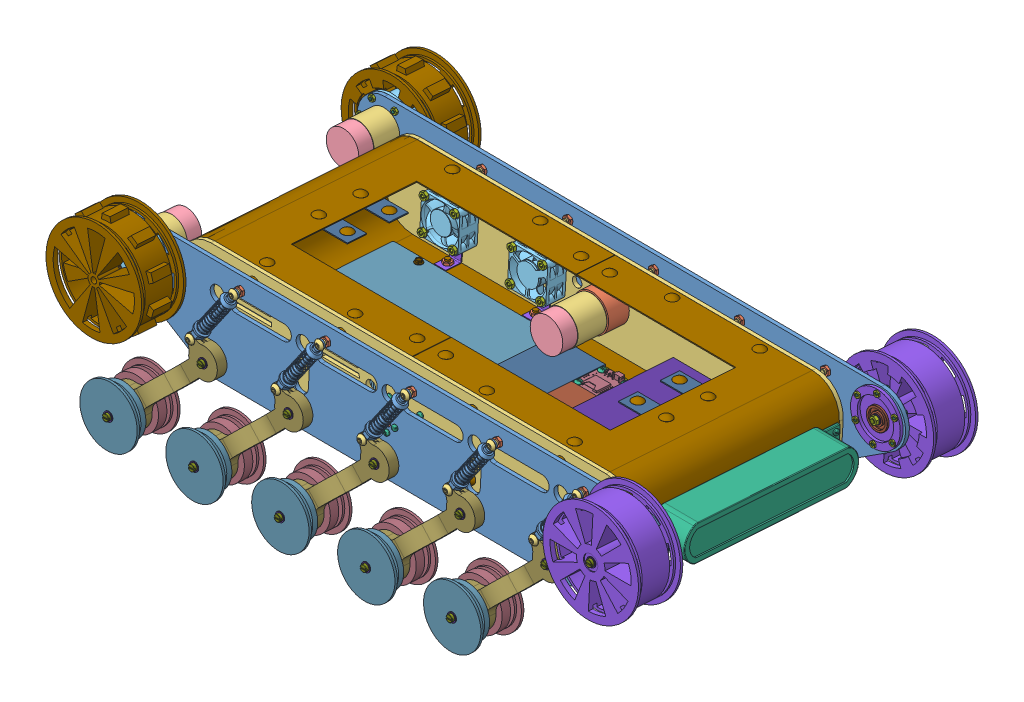
SolidWorks assembly Ensamble_Detallado_2, configuration Predeterminado. Lengths in mm.
Overall size (769.79 225.93 366.19).
522 component instances, 48 part files, 262 mates.
Components (placement in the parent):
- Perfil_IzquierdoV2.2-1: Perfil_IzquierdoV2.2 [Predeterminado] at (68.4496 -9.6253 -539.9326) x (0.999983 -0.000205 0.005895) z (-0.005872 0.060029 0.998179) size (574.48 100.85 4)
- Motor_4-1: Motor_4 [Predeterminado] at (-189.8361 39.4073 -564.1867) x (0.999983 -0.000205 0.005895) z (-0.005872 0.060029 0.998179) size (43.61 43.61 89.6)
  - Motor_1-1: Motor_1 [Predeterminado] at (-1.5658 -18.1483 21.75) size (36.8 36.8 43.5)
  - Motor_2-1: Motor_2 [Predeterminado] at (-1.5658 -18.1483 -8.95) x (-0.954241 0.299039 0) z (0 0 1) size (34.8 34.8 30.7)
  - Motor_3-1: Motor_3 [Predeterminado] at (-1.5658 -18.1483 -24.35) x (0.996313 -0.085794 0) z (0 0 1) size (34 34 15.4)
- Tapa_motor-1: Tapa_motor [Predeterminado] at (-191.6836 24.0684 -516.9408) x (-0.999983 0.000205 -0.005895) z (0.005872 -0.060029 -0.998179) size (54.48 54.48 24.5)
- pan head tapping screw_am-8: pan head tapping screw_am [PHT 3x6x5.5-slot-D-N] at (-183.9391 37.598 -515.5049) x (0.005872 -0.060029 -0.998179) z (-0.134849 -0.989126 0.058691) size (8.2 5.6 5.6)
- pan head tapping screw_am-9: pan head tapping screw_am [PHT 3x6x5.5-slot-D-N] at (-176.1968 24.1972 -514.6534) x (0.005872 -0.060029 -0.998179) z (-0.925525 -0.378291 0.017305) size (8.2 5.6 5.6)
- pan head tapping screw_am-10: pan head tapping screw_am [PHT 3x6x5.5-slot-D-N] at (-183.9541 10.7996 -513.8933) x (0.005872 -0.060029 -0.998179) z (-0.790675 0.610835 -0.041386) size (8.2 5.6 5.6)
- pan head tapping screw_am-11: pan head tapping screw_am [PHT 3x6x5.5-slot-D-N] at (-199.4539 10.8028 -513.9847) x (0.005872 -0.060029 -0.998179) z (0.134849 0.989126 -0.058691) size (8.2 5.6 5.6)
- pan head tapping screw_am-12: pan head tapping screw_am [PHT 3x6x5.5-slot-D-N] at (-207.1962 24.2036 -514.8361) x (0.005872 -0.060029 -0.998179) z (0.925525 0.378291 -0.017305) size (8.2 5.6 5.6)
- pan head tapping screw_am-13: pan head tapping screw_am [PHT 3x6x5.5-slot-D-N] at (-199.4389 37.6012 -515.5962) x (0.005872 -0.060029 -0.998179) z (0.790675 -0.610835 0.041386) size (8.2 5.6 5.6)
- pan head tapping screw_am-14: pan head tapping screw_am [PHT 3x10x9-slot-D-N] at (-215.3099 22.8964 -536.3445) x (0.005872 -0.060029 -0.998179) z (0.809274 0.586638 -0.030519) size (12.2 5.6 5.6)
- hex nut style 1_am-1: hex nut style 1_am [B18.2.4.1M - Hex nut, Style 1,  M3 x 0.5 --D-N] at (-215.2558 22.3441 -545.5277) x (0.970127 -0.241753 0.020245) z (-0.005872 0.060029 0.998179) size (5.5 6.35 2.4)
- Pieza_Fijacion-1: Pieza_Fijacion [Predeterminado] at (328.1431 22.6984 -545.358) x (0.999454 -0.032109 0.00781) z (0.005872 -0.060029 -0.998179) size (52 52 4)
- pan head tapping screw_am-20: pan head tapping screw_am [PHT 3x10x9-slot-D-N] at (328.8149 45.7585 -536.5222) x (0.005872 -0.060029 -0.998179) z (0.852997 -0.520651 0.036329) size (12.2 5.6 5.6)
- hex nut style 1_am-7: hex nut style 1_am [B18.2.4.1M - Hex nut, Style 1,  M3 x 0.5 --D-N] at (328.8748 45.1462 -546.7037) x (-0.437994 -0.897507 0.051398) z (-0.005872 0.060029 0.998179) size (5.5 6.35 2.4)
- Ensamble_internoV1.1-1: Ensamble_internoV1.1 [Predeterminado] at (-380.1452 -33.1767 -776.9821) x (0.005872 -0.060029 -0.998179) z (0.999983 0.000382 0.005859) size (210 91 474)
  - ChasisV1.7-1: ChasisV1.7 [Predeterminado] at (-114.8477 22.7516 450) size (210 84 474)
  - roboclaw-1: roboclaw [Predeterminado] at (-157.9377 -17.2484 439.18) x (1 0 0) z (0 1 0) size (74 52 2)
  - roboclaw-3: roboclaw [Predeterminado] at (-61.7577 -17.2484 439.18) x (-1 0 0) z (0 1 0) size (74 52 2)
  - Regulador-1: Regulador [Predeterminado] at (-109.8477 -17.2484 499.18) x (-1 0 0) z (0 1 0) size (100 68 2)
  - Conmutador-1: Conmutador [Predeterminado] at (-174.0717 -17.2484 490.58) x (0 0 1) z (0 1 0) size (50.8 28.45 2)
  - imu-1: imu [Default] at (-43.9727 -15.9784 481.055) x (-1 0 0) z (0 0 1) size (31.75 5.84 31.75)
  - jetson-1: jetson [Predeterminado] at (-188.5877 -15.6734 408.1) x (1 0 0) z (0 1 0) size (170.18 170.18 1.57)
  - lipo_holder-1: lipo_holder [Predeterminado] at (-109.8477 -18.2484 627) x (0 0 -1) z (0 1 0) size (60 185 60)
  - Plastico-1: Plastico [Predeterminado] at (-109.8477 -18.2484 388.09) x (1 0 0) z (0 1 0) size (170.18 290.18 1)
  - lipo_holder-2: lipo_holder [Predeterminado] at (-109.8477 -18.2484 567) x (0 0 -1) z (0 1 0) size (60 185 60)
  - batería-1: batería [Predeterminado] at (-32.3477 -14.2484 604) x (0 1 0) z (0 0 1) size (48 152 48)
  - batería-2: batería [Predeterminado] at (-35.3477 -14.2484 544) x (0 1 0) z (0 0 1) size (48 152 48)
  - hex flange head tapping screw_am-1: hex flange head tapping screw_am [HEXFHTS 3.5x8x6.7-Indented head-AB-N] at (-31.1077 -15.6734 276.02) x (0 -1 0) z (0 0 1) size (10.9 7.5 7.5)
  - hex flange head tapping screw_am-2: hex flange head tapping screw_am [HEXFHTS 3.5x8x6.7-Indented head-AB-N] at (-188.5877 -15.6734 253.18) x (0 -1 0) z (0 0 1) size (10.9 7.5 7.5)
  - hex flange head tapping screw_am-3: hex flange head tapping screw_am [HEXFHTS 3.5x8x6.7-Indented head-AB-N] at (-188.5877 -15.6734 408.1) x (0 -1 0) z (0 0 1) size (10.9 7.5 7.5)
  - hex flange head tapping screw_am-4: hex flange head tapping screw_am [HEXFHTS 3.5x8x6.7-Indented head-AB-N] at (-31.1077 -15.6734 408.1) x (0 -1 0) z (0 0 1) size (10.9 7.5 7.5)
  - prevailing torque hex nut_am-1: prevailing torque hex nut_am [AM-M3.5-N] at (-31.1077 -22.7484 276.02) x (1 0 0) z (0 -1 0) size (6 7.33 3.5)
  - prevailing torque hex nut_am-2: prevailing torque hex nut_am [AM-M3.5-N] at (-188.5877 -22.7484 253.18) x (1 0 0) z (0 -1 0) size (6 7.33 3.5)
  - prevailing torque hex nut_am-3: prevailing torque hex nut_am [AM-M3.5-N] at (-31.1077 -22.7484 408.1) x (1 0 0) z (0 -1 0) size (6 7.33 3.5)
  - prevailing torque hex nut_am-4: prevailing torque hex nut_am [AM-M3.5-N] at (-188.5877 -22.7484 408.1) x (0.006529 0 -0.999979) z (0 -1 0) size (6 7.33 3.5)
  - pan head tapping screw_am-1: pan head tapping screw_am [PHT 4.2x8x6.6-slot-AB-N] at (-31.7377 -14.1484 493.29) x (0 -1 0) z (0 0 1) size (11.21 7 7)
  - pan head tapping screw_am-2: pan head tapping screw_am [PHT 4.2x8x6.6-slot-AB-N] at (-56.2081 -15.1484 493.2904) x (0 -1 0) z (0 0 1) size (11.21 7 7)
  - pan head tapping screw_am-4: pan head tapping screw_am [PHT 4.2x8x6.6-slot-AB-N] at (-56.2077 -14.1484 468.82) x (0 -1 0) z (0 0 1) size (11.21 7 7)
  - pan head tapping screw_am-5: pan head tapping screw_am [PHT 4.2x8x6.6-slot-AB-N] at (-31.7377 -14.1484 468.82) x (0 -1 0) z (0 0 1) size (11.21 7 7)
  - hex nut jam_am-3: hex nut jam_am [B18.2.4.5M - Hex jam nut,  M5 x 0.8 --D-N] at (-31.7377 -19.2484 493.29) x (0.998096 0 -0.061678) z (0 1 0) size (8 9.24 2.7)
  - hex nut jam_am-4: hex nut jam_am [B18.2.4.5M - Hex jam nut,  M5 x 0.8 --D-N] at (-56.2081 -21.9484 493.2904) x (0 0 -1) z (0 -1 0) size (8 9.24 2.7)
  - hex nut jam_am-5: hex nut jam_am [B18.2.4.5M - Hex jam nut,  M5 x 0.8 --D-N] at (-31.7377 -21.9484 468.82) x (1 0 0) z (0 -1 0) size (8 9.24 2.7)
  - hex nut jam_am-6: hex nut jam_am [B18.2.4.5M - Hex jam nut,  M5 x 0.8 --D-N] at (-56.2077 -21.9484 468.82) x (0 0 -1) z (0 -1 0) size (8 9.24 2.7)
  - socket button head cap screw_am-3: socket button head cap screw_am [B18.3.4M - 4 x 0.7 x 8 SBHCS --N] at (-22.3477 -12.0484 617) x (0 -1 0) z (-0.458504 0 0.888692) size (10.2 7.6 7.6)
  - socket button head cap screw_am-4: socket button head cap screw_am [B18.3.4M - 4 x 0.7 x 8 SBHCS --N] at (-22.3477 -12.0484 557) x (0 -1 0) z (-0.211914 0 0.977288) size (10.2 7.6 7.6)
  - socket button head cap screw_am-5: socket button head cap screw_am [B18.3.4M - 4 x 0.7 x 8 SBHCS --N] at (-22.3477 -12.0484 576.6022) x (0 -1 0) z (-0.545234 0 0.838284) size (10.2 7.6 7.6)
  - socket button head cap screw_am-6: socket button head cap screw_am [B18.3.4M - 4 x 0.7 x 8 SBHCS --N] at (-22.3477 -12.0484 636.6022) x (0 -1 0) z (-0.646269 0 0.76311) size (10.2 7.6 7.6)
  - hex thin nut gradeb_din-1: hex thin nut gradeb_din [Hexagon Nut ISO 4036 - M4 - N] at (-22.3477 -19.4976 636.6022) x (1 0 0) z (0 1 0) size (7 8.08 2.2)
  - hex thin nut gradeb_din-2: hex thin nut gradeb_din [Hexagon Nut ISO 4036 - M4 - N] at (-22.3477 -19.6363 617) x (1 0 0) z (0 1 0) size (7 8.08 2.2)
  - hex thin nut gradeb_din-3: hex thin nut gradeb_din [Hexagon Nut ISO 4036 - M4 - N] at (-147.9786 -8.1538 555.9748) size (7 8.08 2.2)
  - hex thin nut gradeb_din-4: hex thin nut gradeb_din [Hexagon Nut ISO 4036 - M4 - N] at (-22.3477 -21.4484 557) x (-0.957833 0 0.287325) z (0 -1 0) size (7 8.08 2.2)
  - hex thin nut gradeb_din-5: hex thin nut gradeb_din [Hexagon Nut ISO 4036 - M4 - N] at (-22.3477 -19.2484 576.6022) x (0.99798 0 0.063529) z (0 1 0) size (7 8.08 2.2)
  - socket button head cap screw_am-8: socket button head cap screw_am [B18.3.4M - 4 x 0.7 x 8 SBHCS --N] at (-197.3477 -12.0484 557) x (0 -1 0) z (-0.211914 0 -0.977288) size (10.2 7.6 7.6)
  - socket button head cap screw_am-9: socket button head cap screw_am [B18.3.4M - 4 x 0.7 x 8 SBHCS --N] at (-197.3477 -12.0484 576.6022) x (0 -1 0) z (-0.545234 0 -0.838284) size (10.2 7.6 7.6)
  - socket button head cap screw_am-10: socket button head cap screw_am [B18.3.4M - 4 x 0.7 x 8 SBHCS --N] at (-197.3477 -12.0484 617) x (0 -1 0) z (-0.458504 0 -0.888692) size (10.2 7.6 7.6)
  - socket button head cap screw_am-11: socket button head cap screw_am [B18.3.4M - 4 x 0.7 x 8 SBHCS --N] at (-197.3477 -12.0484 636.6022) x (0 -1 0) z (-0.646269 0 -0.76311) size (10.2 7.6 7.6)
  - hex thin nut gradeb_din-6: hex thin nut gradeb_din [Hexagon Nut ISO 4036 - M4 - N] at (-197.3477 -21.4484 576.6022) x (-0.99798 0 0.063529) z (0 -1 0) size (7 8.08 2.2)
  - hex thin nut gradeb_din-7: hex thin nut gradeb_din [Hexagon Nut ISO 4036 - M4 - N] at (-197.3477 -19.2484 557) x (0.957833 0 0.287325) z (0 1 0) size (7 8.08 2.2)
  - hex thin nut gradeb_din-8: hex thin nut gradeb_din [Hexagon Nut ISO 4036 - M4 - N] at (-197.3477 -21.8363 617) x (-1 0 0) z (0 -1 0) size (7 8.08 2.2)
  - hex thin nut gradeb_din-9: hex thin nut gradeb_din [Hexagon Nut ISO 4036 - M4 - N] at (-197.3477 -21.6976 636.6022) x (-1 0 0) z (0 -1 0) size (7 8.08 2.2)
- fan-1: fan [По умолчанию] at (0.0753 3.2018 -561.6937) x (-0.999983 -0.000176 -0.005872) z (0.005872 -0.060029 -0.998179) size (41.13 41.33 20.18)
- fan-2: fan [По умолчанию] at (-91.8057 2.0201 -582.1996) x (0.999983 0.000176 0.005872) z (-0.005872 0.060029 0.998179) size (41.13 41.33 20.18)
- Soporte_zed-1: Soporte_zed [Predeterminado] at (340.1967 -3.5969 -664.4756) x (-0.005872 0.060029 0.998179) z (-0.999983 -0.000382 -0.005859) size (205.99 36.47 36.01)
- hex nut style 1 gradeab_bsi-1: hex nut style 1 gradeab_bsi [BS EN 24032 - M4 - W - N] at (-107.8026 17.9884 -583.254) x (0.99528 -0.096345 0.011649) z (-0.005872 0.060029 0.998179) size (7 8.08 3.2)
- hex nut style 1 gradeab_bsi-2: hex nut style 1 gradeab_bsi [BS EN 24032 - M4 - W - N] at (-107.7894 -14.1459 -584.5273) x (-0.581467 -0.8123 0.04543) z (0.005872 -0.060029 -0.998179) size (7 8.08 3.2)
- hex nut style 1 gradeab_bsi-3: hex nut style 1 gradeab_bsi [BS EN 24032 - M4 - W - N] at (-75.79 -14.1403 -584.3394) x (-0.984097 0.176868 -0.016425) z (0.005872 -0.060029 -0.998179) size (7 8.08 3.2)
- hex nut style 1 gradeab_bsi-4: hex nut style 1 gradeab_bsi [BS EN 24032 - M4 - W - N] at (-75.7843 17.802 -586.2603) x (-0.58545 0.809033 -0.052098) z (0.005872 -0.060029 -0.998179) size (7 8.08 3.2)
- hex nut style 1 gradeab_bsi-5: hex nut style 1 gradeab_bsi [BS EN 24032 - M4 - W - N] at (-15.7854 17.7775 -585.9059) x (-0.58545 0.809033 -0.052098) z (0.005872 -0.060029 -0.998179) size (7 8.08 3.2)
- hex nut style 1 gradeab_bsi-6: hex nut style 1 gradeab_bsi [BS EN 24032 - M4 - W - N] at (-15.791 -14.1648 -583.985) x (0.609484 0.791576 -0.044019) z (0.005872 -0.060029 -0.998179) size (7 8.08 3.2)
- hex nut style 1 gradeab_bsi-7: hex nut style 1 gradeab_bsi [BS EN 24032 - M4 - W - N] at (16.2141 17.7832 -585.718) x (-0.984097 0.176868 -0.016425) z (0.005872 -0.060029 -0.998179) size (7 8.08 3.2)
- hex nut style 1 gradeab_bsi-8: hex nut style 1 gradeab_bsi [BS EN 24032 - M4 - W - N] at (16.2084 -14.1591 -583.7971) x (0.609484 0.791576 -0.044019) z (0.005872 -0.060029 -0.998179) size (7 8.08 3.2)
- Pieza_union_chasis-1: Pieza_union_chasis [Predeterminado] at (-92.4935 43.6291 -564.6695) x (-0.999983 -0.000382 -0.005859) z (0.005872 -0.060029 -0.998179) size (12 20 17)
- round head bolt_ai-8: round head bolt_ai [RHBOLT 0.19-24x0.25x0.25-N] at (-92.3708 46.562 -573.8615) x (0.000029 -0.998197 0.06003) z (-0.000001 0.06003 0.998197) size (8.99 11.53 11.53)
- hex nut jam_am-6: hex nut jam_am [B18.2.4.5M - Hex jam nut,  M5 x 0.8 --D-N] at (-92.3707 42.0907 -573.5926) x (0.997706 0.004093 0.067568) z (-0.000029 0.998197 -0.06003) size (8 9.24 2.7)
- round head bolt_ai-9: round head bolt_ai [RHBOLT 0.19-24x0.25x0.25-N] at (-92.5322 32.0495 -557.3196) x (0.005872 -0.060029 -0.998179) z (0 -0.998197 0.06003) size (8.99 11.53 11.53)
- hex nut jam_am-7: hex nut jam_am [B18.2.4.5M - Hex jam nut,  M5 x 0.8 --D-N] at (-92.4715 31.4287 -567.6424) x (0.997689 0.06792 0.001784) z (0.005872 -0.060029 -0.998179) size (8 9.24 2.7)
- hex nut jam_am-10: hex nut jam_am [B18.2.4.5M - Hex jam nut,  M5 x 0.8 --D-N] at (-0.3831 31.4638 -567.1028) x (0.997689 0.06792 0.001784) z (0.005872 -0.060029 -0.998179) size (8 9.24 2.7)
- round head bolt_ai-12: round head bolt_ai [RHBOLT 0.19-24x0.25x0.25-N] at (-0.4438 32.0846 -556.78) x (0.005872 -0.060029 -0.998179) z (0 -0.998197 0.06003) size (8.99 11.53 11.53)
- Pieza_union_chasis-3: Pieza_union_chasis [Predeterminado] at (-0.4051 43.6643 -564.1299) x (-0.999983 -0.000382 -0.005859) z (0.005872 -0.060029 -0.998179) size (12 20 17)
- round head bolt_ai-13: round head bolt_ai [RHBOLT 0.19-24x0.25x0.25-N] at (-0.2824 46.5972 -573.3219) x (0.000029 -0.998197 0.06003) z (-0.000001 0.06003 0.998197) size (8.99 11.53 11.53)
- hex nut jam_am-11: hex nut jam_am [B18.2.4.5M - Hex jam nut,  M5 x 0.8 --D-N] at (-0.2823 42.1259 -573.0531) x (0.997706 0.004093 0.067568) z (-0.000029 0.998197 -0.06003) size (8 9.24 2.7)
- Pieza_union_chasis-4: Pieza_union_chasis [Predeterminado] at (137.5925 43.636 -563.3164) x (-0.999983 -0.000382 -0.005859) z (0.005872 -0.060029 -0.998179) size (12 20 17)
- round head bolt_ai-14: round head bolt_ai [RHBOLT 0.19-24x0.25x0.25-N] at (137.5538 32.0564 -555.9666) x (0.005872 -0.060029 -0.998179) z (0 -0.998197 0.06003) size (8.99 11.53 11.53)
- hex nut jam_am-12: hex nut jam_am [B18.2.4.5M - Hex jam nut,  M5 x 0.8 --D-N] at (137.6145 31.4356 -566.2893) x (0.997689 0.06792 0.001784) z (0.005872 -0.060029 -0.998179) size (8 9.24 2.7)
- round head bolt_ai-15: round head bolt_ai [RHBOLT 0.19-24x0.25x0.25-N] at (137.7152 46.5689 -572.5085) x (0.000029 -0.998197 0.06003) z (-0.000001 0.06003 0.998197) size (8.99 11.53 11.53)
- hex nut jam_am-13: hex nut jam_am [B18.2.4.5M - Hex jam nut,  M5 x 0.8 --D-N] at (137.7153 42.0976 -572.2396) x (0.997706 0.004093 0.067568) z (-0.000029 0.998197 -0.06003) size (8 9.24 2.7)
- Puerta-1: Puerta [Predeterminado] at (69.2002 37.2257 -668.5247) x (0.005872 -0.060029 -0.998179) z (-0.000029 0.998197 -0.06003) size (130 334 1) (hidden)
- lamina_union-2: lamina_union [Predeterminado] at (236.0701 38.5901 -645.919) x (-0.005872 0.060029 0.998179) z (0.000029 -0.998197 0.06003) size (20 50 1)
- lamina_union-3: lamina_union [Predeterminado] at (68.7011 41.33 -583.6195) x (0.005872 -0.060029 -0.998179) z (-0.000029 0.998197 -0.06003) size (20 50 1)
- lamina_union-4: lamina_union [Predeterminado] at (-97.9242 38.4626 -647.876) x (-0.005872 0.060029 0.998179) z (0.000029 -0.998197 0.06003) size (20 50 1)
- round head bolt_ai-26: round head bolt_ai [RHBOLT 0.19-24x0.25x0.25-N] at (-112.924 42.0919 -648.1825) x (0.000029 -0.998197 0.06003) z (-0.000001 0.06003 0.998197) size (8.99 11.53 11.53)
- hex nut jam_am-24: hex nut jam_am [B18.2.4.5M - Hex jam nut,  M5 x 0.8 --D-N] at (251.0698 37.5976 -645.7711) x (0.997706 0.004093 0.067568) z (-0.000029 0.998197 -0.06003) size (8 9.24 2.7)
- round head bolt_ai-27: round head bolt_ai [RHBOLT 0.19-24x0.25x0.25-N] at (-82.9245 42.1033 -648.0067) x (0.000029 -0.998197 0.06003) z (-0.000001 0.06003 0.998197) size (8.99 11.53 11.53)
- round head bolt_ai-28: round head bolt_ai [RHBOLT 0.19-24x0.25x0.25-N] at (83.7007 45.9689 -583.8102) x (0.000029 -0.998197 0.06003) z (-0.000001 0.06003 0.998197) size (8.99 11.53 11.53)
- round head bolt_ai-29: round head bolt_ai [RHBOLT 0.19-24x0.25x0.25-N] at (221.0702 42.2194 -646.2255) x (0.000029 -0.998197 0.06003) z (-0.000001 0.06003 0.998197) size (8.99 11.53 11.53)
- round head bolt_ai-30: round head bolt_ai [RHBOLT 0.19-24x0.25x0.25-N] at (251.0697 42.2309 -646.0497) x (0.000029 -0.998197 0.06003) z (-0.000001 0.06003 0.998197) size (8.99 11.53 11.53)
- round head bolt_ai-31: round head bolt_ai [RHBOLT 0.19-24x0.25x0.25-N] at (53.7012 45.9575 -583.986) x (0.000029 -0.998197 0.06003) z (-0.000001 0.06003 0.998197) size (8.99 11.53 11.53)
- hex nut jam_am-25: hex nut jam_am [B18.2.4.5M - Hex jam nut,  M5 x 0.8 --D-N] at (-112.9239 37.4586 -647.9039) x (0.924389 -0.022871 -0.380764) z (-0.000029 0.998197 -0.06003) size (8 9.24 2.7)
- hex nut jam_am-26: hex nut jam_am [B18.2.4.5M - Hex jam nut,  M5 x 0.8 --D-N] at (83.7008 41.3357 -583.5316) x (0.642396 -0.045986 -0.764992) z (-0.000029 0.998197 -0.06003) size (8 9.24 2.7)
- hex nut jam_am-27: hex nut jam_am [B18.2.4.5M - Hex jam nut,  M5 x 0.8 --D-N] at (53.7014 41.3242 -583.7074) x (0.987847 0.00936 0.155149) z (-0.000029 0.998197 -0.06003) size (8 9.24 2.7)
- hex nut jam_am-28: hex nut jam_am [B18.2.4.5M - Hex jam nut,  M5 x 0.8 --D-N] at (221.0704 37.5862 -645.9469) x (0.944813 0.019694 0.327016) z (-0.000029 0.998197 -0.06003) size (8 9.24 2.7)
- hex nut jam_am-29: hex nut jam_am [B18.2.4.5M - Hex jam nut,  M5 x 0.8 --D-N] at (-82.9244 37.4701 -647.7281) x (0.961929 0.016435 0.272807) z (-0.000029 0.998197 -0.06003) size (8 9.24 2.7)
- instrument ball bearing_68_am-5: instrument ball bearing_68_am [AFBMA 12.1.4.1 - 0080-22 - 8,SI,NC,8_68] at (188.8254 -92.4717 -505.6903) x (0.005872 -0.060029 -0.998179) z (0.436634 -0.897859 0.056564) size (7 22 22)
- Pieza_ResorteV1.5-6: Pieza_ResorteV1.5 [Predeterminado] at (188.8254 -92.4717 -505.6903) x (-0.005872 0.060029 0.998179) z (-0.699298 -0.713776 0.038812) size (30 44.97 120)
- Rueda_Resorte2V1.3-13: Rueda_Resorte2V1.3 [Predeterminado] at (188.8548 -92.7718 -510.6812) x (-0.998179 -0.060274 -0.002247) z (0.005872 -0.060029 -0.998179) size (60 60 20.5)
- Rueda_ResorteV1.3-17: Rueda_ResorteV1.3 [Predeterminado] at (188.7961 -92.1715 -500.6994) x (-0.99968 0.024219 -0.007337) z (-0.005872 0.060029 0.998179) size (60 60 17)
- Pasador-1: Pasador [Predeterminado] at (188.9664 -93.9124 -529.6466) x (0.998179 0.060274 0.002247) z (-0.005872 0.060029 0.998179) size (8 8 44.5)
- cheese head screw_as-2: cheese head screw_as [AS-NZS 1427 CH - M4 x 50-N] at (188.6851 -91.037 -481.8338) x (0.005872 -0.060029 -0.998179) z (-0.998179 -0.060274 -0.002247) size (52.62 7 7)
- plain washer - normal_as-1: plain washer - normal_as [AS 1237.1 N - 4] at (188.9711 -93.9604 -530.4452) x (-0.998179 -0.060274 -0.002247) z (0.005872 -0.060029 -0.998179) size (9 9 0.8)
- hex nut style 1_am-62: hex nut style 1_am [B18.2.4.1M - Hex nut, Style 1,  M4 x 0.7 --D-N] at (188.9899 -94.1525 -533.6393) x (-0.998179 -0.060274 -0.002247) z (0.005872 -0.060029 -0.998179) size (7 8.08 3.2)
- plain washer - normal_as-2: plain washer - normal_as [AS 1237.1 N - 4] at (188.7051 -91.2411 -485.2276) x (-0.998179 -0.060274 -0.002247) z (0.005872 -0.060029 -0.998179) size (9 9 0.8)
- Pieza_Resorte_2V1.5-1: Pieza_Resorte_2V1.5 [Predeterminado] at (190.6345 -110.9665 -813.2294) x (0.005872 -0.060029 -0.998179) z (-0.699298 -0.713776 0.038812) size (30 44.97 120)
- cheese head screw_as-3: cheese head screw_as [AS-NZS 1427 CH - M4 x 50-N] at (190.7748 -112.4012 -837.0859) x (-0.005872 0.060029 0.998179) z (-0.99997 -0.005414 -0.005557) size (52.62 7 7)
- hex nut style 1_am-63: hex nut style 1_am [B18.2.4.1M - Hex nut, Style 1,  M4 x 0.7 --D-N] at (190.4889 -109.4778 -788.4745) x (-0.99997 -0.005414 -0.005557) z (0.005872 -0.060029 -0.998179) size (7 8.08 3.2)
- plain washer - normal_as-3: plain washer - normal_as [AS 1237.1 N - 4] at (190.4936 -109.5258 -789.2731) x (-0.99997 -0.005414 -0.005557) z (0.005872 -0.060029 -0.998179) size (9 9 0.8)
- Pasador-2: Pasador [Predeterminado] at (190.7549 -112.1971 -833.692) x (0.999795 0.019701 0.004696) z (-0.005872 0.060029 0.998179) size (8 8 44.5)
- instrument ball bearing_68_am-6: instrument ball bearing_68_am [AFBMA 12.1.4.1 - 0080-22 - 8,SI,NC,8_68] at (190.6345 -110.9665 -813.2294) x (0.005872 -0.060029 -0.998179) z (0.386524 -0.920477 0.05763) size (7 22 22)
- plain washer - normal_as-4: plain washer - normal_as [AS 1237.1 N - 4] at (190.7596 -112.2451 -834.4906) x (-0.99997 -0.005414 -0.005557) z (0.005872 -0.060029 -0.998179) size (9 9 0.8)
- instrument ball bearing_68_am-7: instrument ball bearing_68_am [AFBMA 12.1.4.1 - 0080-22 - 8,SI,NC,8_68] at (249.9398 -48.9149 -793.5702) x (-0.005872 0.060029 0.998179) z (-0.454454 -0.88932 0.050809) size (7 22 22)
- Resorte-1: Resorte [Predeterminado] at (241.4602 -8.2795 -530.4803) x (-0.827134 0.560678 -0.038584) z (-0.561974 -0.825855 0.04636) size (14 14 75.95)
- Resorte-2: Resorte [Predeterminado] at (243.0344 -24.3732 -798.0922) x (-0.827134 0.560678 -0.038584) z (-0.561974 -0.825855 0.04636) size (14 14 75.95)
- socket button head cap screw_am-5: socket button head cap screw_am [B18.3.4M - 5 x 0.8 x 10 SBHCS --N] at (235.7742 -35.5745 -805.2254) x (-0.005872 0.060029 0.998179) z (-0.100585 -0.993169 0.059136) size (12.75 9.5 9.5)
- socket button head cap screw_am-6: socket button head cap screw_am [B18.3.4M - 5 x 0.8 x 10 SBHCS --N] at (234.109 -18.5503 -522.1418) x (0.005872 -0.060029 -0.998179) z (-0.163306 0.984738 -0.060181) size (12.75 9.5 9.5)
- Motor_4-2: Motor_4 [Predeterminado] at (67.8778 18.2739 -605.5302) x (0.994997 0.099904 -0.000155) z (-0.005872 0.060029 0.998179) size (43.61 43.61 89.6)
  - Motor_1-1: Motor_1 [Predeterminado] at (-1.5658 -18.1483 21.75) size (36.8 36.8 43.5)
  - Motor_2-1: Motor_2 [Predeterminado] at (-1.5658 -18.1483 -8.95) x (-0.954241 0.299039 0) z (0 0 1) size (34.8 34.8 30.7)
  - Motor_3-1: Motor_3 [Predeterminado] at (-1.5658 -18.1483 -24.35) x (0.996313 -0.085794 0) z (0 0 1) size (34 34 15.4)
- Acople-1: Acople [Predeterminado] at (68.465 -3.1497 -542.3256) x (0.999983 -0.000205 0.005895) z (0.005872 -0.060029 -0.998179) size (22 22 12)
- Pared_chasis-2: Pared_chasis [Predeterminado] at (68.5756 -1.2687 -561.0219) x (0.999983 -0.000205 0.005895) z (-0.005872 0.060029 0.998179) size (474 84 4)
- pan head tapping screw_am-43: pan head tapping screw_am [PHT 3x10x9-slot-D-N] at (76.0451 16.9329 -555.8613) x (0.005872 -0.060029 -0.998179) z (-0.866854 -0.497942 0.024846) size (12.2 5.6 5.6)
- pan head tapping screw_am-44: pan head tapping screw_am [PHT 3x10x9-slot-D-N] at (76.4285 -2.7792 -536.0897) x (0.005872 -0.060029 -0.998179) z (-0.866854 -0.497942 0.024846) size (12.2 5.6 5.6)
- pan head tapping screw_am-45: pan head tapping screw_am [PHT 3x10x9-slot-D-N] at (59.91 17.0865 -555.9654) x (0.005872 -0.060029 -0.998179) z (-0.00169 -0.998196 0.06002) size (12.2 5.6 5.6)
- pan head tapping screw_am-46: pan head tapping screw_am [PHT 3x10x9-slot-D-N] at (51.7043 3.2148 -555.1795) x (0.005872 -0.060029 -0.998179) z (0.865164 -0.500253 0.035174) size (12.2 5.6 5.6)
- pan head tapping screw_am-47: pan head tapping screw_am [PHT 3x10x9-slot-D-N] at (59.6337 -10.8105 -554.2894) x (0.005872 -0.060029 -0.998179) z (0.866854 0.497942 -0.024846) size (12.2 5.6 5.6)
- pan head tapping screw_am-48: pan head tapping screw_am [PHT 3x10x9-slot-D-N] at (75.7688 -10.9641 -554.1852) x (0.005872 -0.060029 -0.998179) z (0.00169 0.998196 -0.06002) size (12.2 5.6 5.6)
- pan head tapping screw_am-49: pan head tapping screw_am [PHT 3x10x9-slot-D-N] at (83.9745 2.9076 -554.9712) x (0.005872 -0.060029 -0.998179) z (-0.865164 0.500253 -0.035174) size (12.2 5.6 5.6)
- pan head tapping screw_am-50: pan head tapping screw_am [PHT 3x10x9-slot-D-N] at (68.4331 5.208 -536.6171) x (0.005872 -0.060029 -0.998179) z (0.498527 -0.86513 0.05496) size (12.2 5.6 5.6)
- pan head tapping screw_am-51: pan head tapping screw_am [PHT 3x10x9-slot-D-N] at (60.4287 -2.7759 -536.1841) x (0.005872 -0.060029 -0.998179) z (0.866854 0.497942 -0.024846) size (12.2 5.6 5.6)
- pan head tapping screw_am-52: pan head tapping screw_am [PHT 3x10x9-slot-D-N] at (68.4241 -10.7631 -535.6567) x (0.005872 -0.060029 -0.998179) z (-0.498527 0.86513 -0.05496) size (12.2 5.6 5.6)
- hex nut style 1_am-64: hex nut style 1_am [B18.2.4.1M - Hex nut, Style 1,  M3 x 0.5 --D-N] at (76.4766 -3.2714 -544.2748) x (-0.695099 -0.717851 0.039081) z (-0.005872 0.060029 0.998179) size (5.5 6.35 2.4)
- hex nut style 1_am-65: hex nut style 1_am [B18.2.4.1M - Hex nut, Style 1,  M3 x 0.5 --D-N] at (68.4723 -11.2554 -543.8418) x (-0.71889 0.693604 -0.045941) z (-0.005872 0.060029 0.998179) size (5.5 6.35 2.4)
- hex nut style 1_am-66: hex nut style 1_am [B18.2.4.1M - Hex nut, Style 1,  M3 x 0.5 --D-N] at (60.4769 -3.2681 -544.3691) x (0.695099 0.717851 -0.039081) z (-0.005872 0.060029 0.998179) size (5.5 6.35 2.4)
- hex nut style 1_am-67: hex nut style 1_am [B18.2.4.1M - Hex nut, Style 1,  M3 x 0.5 --D-N] at (68.4812 4.7158 -544.8022) x (0.71889 -0.693604 0.045941) z (-0.005872 0.060029 0.998179) size (5.5 6.35 2.4)
- socket set screw cup point_ai-2: socket set screw cup point_ai [SSCUPSKT 0.125-44x0.125-HX-N] at (68.5089 1.4211 -549.613) x (-0.000558 -0.998197 0.060026) z (-0.47589 0.053059 0.877903) size (3.17 3.17 3.17)
- round head bolt_ai-32: round head bolt_ai [RHBOLT 0.19-24x0.25x0.25-N] at (229.6436 46.685 -571.9747) x (0.000029 -0.998197 0.06003) z (-0.000001 0.06003 0.998197) size (8.99 11.53 11.53)
- hex nut jam_am-32: hex nut jam_am [B18.2.4.5M - Hex jam nut,  M5 x 0.8 --D-N] at (229.6437 42.0787 -571.6977) x (0.997706 0.004093 0.067568) z (-0.000029 0.998197 -0.06003) size (8 9.24 2.7)
- hex nut jam_am-33: hex nut jam_am [B18.2.4.5M - Hex jam nut,  M5 x 0.8 --D-N] at (229.6129 31.4167 -565.747) x (0.997689 0.06792 0.001784) z (0.005872 -0.060029 -0.998179) size (8 9.24 2.7)
- round head bolt_ai-33: round head bolt_ai [RHBOLT 0.19-24x0.25x0.25-N] at (229.5522 32.0375 -555.4242) x (0.005872 -0.060029 -0.998179) z (0 -0.998197 0.06003) size (8.99 11.53 11.53)
- Pieza_union_chasis-7: Pieza_union_chasis [Predeterminado] at (229.5909 43.6172 -562.7741) x (-0.999983 -0.000382 -0.005859) z (0.005872 -0.060029 -0.998179) size (12 20 17)
- round head bolt_ai-34: round head bolt_ai [RHBOLT 0.19-24x0.25x0.25-N] at (137.7178 -42.3913 -567.1586) x (-0.000029 0.998197 -0.06003) z (0.000001 -0.06003 -0.998197) size (8.99 11.53 11.53)
- round head bolt_ai-35: round head bolt_ai [RHBOLT 0.19-24x0.25x0.25-N] at (229.6462 -42.4372 -566.615) x (-0.000029 0.998197 -0.06003) z (0.000001 -0.06003 -0.998197) size (8.99 11.53 11.53)
- round head bolt_ai-36: round head bolt_ai [RHBOLT 0.19-24x0.25x0.25-N] at (-92.3682 -42.5602 -568.5019) x (-0.000029 0.998197 -0.06003) z (0.000001 -0.06003 -0.998197) size (8.99 11.53 11.53)
- round head bolt_ai-37: round head bolt_ai [RHBOLT 0.19-24x0.25x0.25-N] at (-0.2798 -42.525 -567.9623) x (-0.000029 0.998197 -0.06003) z (0.000001 -0.06003 -0.998197) size (8.99 11.53 11.53)
- round head bolt_ai-38: round head bolt_ai [RHBOLT 0.19-24x0.25x0.25-N] at (-92.5305 -26.1698 -553.8184) x (0.005872 -0.060029 -0.998179) z (0.000059 -0.998197 0.06003) size (8.99 11.53 11.53)
- round head bolt_ai-39: round head bolt_ai [RHBOLT 0.19-24x0.25x0.25-N] at (-0.4421 -26.1346 -553.2788) x (0.005872 -0.060029 -0.998179) z (0.000059 -0.998197 0.06003) size (8.99 11.53 11.53)
- round head bolt_ai-40: round head bolt_ai [RHBOLT 0.19-24x0.25x0.25-N] at (137.5555 -26.001 -552.4751) x (0.005872 -0.060029 -0.998179) z (0.000059 -0.998197 0.06003) size (8.99 11.53 11.53)
- round head bolt_ai-41: round head bolt_ai [RHBOLT 0.19-24x0.25x0.25-N] at (229.5539 -25.9118 -551.9393) x (0.005872 -0.060029 -0.998179) z (0.000059 -0.998197 0.06003) size (8.99 11.53 11.53)
- Pieza_union_chasis-8: Pieza_union_chasis [Predeterminado] at (-92.4911 -38.5468 -559.7275) x (0.999983 0.000382 0.005859) z (0.005872 -0.060029 -0.998179) size (12 20 17)
- hex nut jam_am-34: hex nut jam_am [B18.2.4.5M - Hex jam nut,  M5 x 0.8 --D-N] at (-92.3684 -35.3937 -568.9328) x (0.997706 0.004093 0.067568) z (-0.000029 0.998197 -0.06003) size (8 9.24 2.7)
- hex nut jam_am-35: hex nut jam_am [B18.2.4.5M - Hex jam nut,  M5 x 0.8 --D-N] at (-92.4856 -26.6285 -561.4461) x (0.997693 -0.067158 0.009908) z (-0.005872 0.060029 0.998179) size (8 9.24 2.7)
- hex nut jam_am-36: hex nut jam_am [B18.2.4.5M - Hex jam nut,  M5 x 0.8 --D-N] at (-0.28 -35.3586 -568.3933) x (0.997706 0.004093 0.067568) z (-0.000029 0.998197 -0.06003) size (8 9.24 2.7)
- Pieza_union_chasis-9: Pieza_union_chasis [Predeterminado] at (-0.4027 -38.5117 -559.1879) x (0.999983 0.000382 0.005859) z (0.005872 -0.060029 -0.998179) size (12 20 17)
- hex nut jam_am-37: hex nut jam_am [B18.2.4.5M - Hex jam nut,  M5 x 0.8 --D-N] at (-0.3972 -26.5933 -560.9065) x (0.997693 -0.067158 0.009908) z (-0.005872 0.060029 0.998179) size (8 9.24 2.7)
- Pieza_union_chasis-10: Pieza_union_chasis [Predeterminado] at (137.5949 -38.378 -558.3842) x (0.999983 0.000382 0.005859) z (0.005872 -0.060029 -0.998179) size (12 20 17)
- hex nut jam_am-38: hex nut jam_am [B18.2.4.5M - Hex jam nut,  M5 x 0.8 --D-N] at (137.7176 -35.2249 -567.5895) x (0.997706 0.004093 0.067568) z (-0.000029 0.998197 -0.06003) size (8 9.24 2.7)
- hex nut jam_am-39: hex nut jam_am [B18.2.4.5M - Hex jam nut,  M5 x 0.8 --D-N] at (137.6004 -26.4597 -560.1028) x (0.997693 -0.067158 0.009908) z (-0.005872 0.060029 0.998179) size (8 9.24 2.7)
- hex nut jam_am-40: hex nut jam_am [B18.2.4.5M - Hex jam nut,  M5 x 0.8 --D-N] at (229.646 -35.1358 -567.0541) x (0.997706 0.004093 0.067568) z (-0.000029 0.998197 -0.06003) size (8 9.24 2.7)
- Pieza_union_chasis-11: Pieza_union_chasis [Predeterminado] at (229.5933 -38.2889 -557.8484) x (0.999983 0.000382 0.005859) z (0.005872 -0.060029 -0.998179) size (12 20 17)
- hex nut jam_am-41: hex nut jam_am [B18.2.4.5M - Hex jam nut,  M5 x 0.8 --D-N] at (229.5988 -26.3706 -559.567) x (0.997693 -0.067158 0.009908) z (-0.005872 0.060029 0.998179) size (8 9.24 2.7)
- pan head tapping screw_am-54: pan head tapping screw_am [PHT 3x10x9-slot-D-N] at (311.9758 -16.5081 -762.5448) x (-0.999983 -0.000382 -0.005859) z (0.005316 -0.482786 -0.875722) size (12.2 5.6 5.6)
- pan head tapping screw_am-55: pan head tapping screw_am [PHT 3x10x9-slot-D-N] at (311.9754 -2.5333 -763.3853) x (-0.999983 -0.000382 -0.005859) z (0.005316 -0.482786 -0.875722) size (12.2 5.6 5.6)
- ZED.step-3: ZED.step [Predeterminado] at (306.0973 -3.6099 -664.6754) x (0.005872 -0.060029 -0.998179) z (0.999983 0.000382 0.005859) size (175 30.01 41.5)
- Tapazed-1: Tapazed [Predeterminado] at (340.5967 -3.5967 -664.4733) x (-0.005872 0.060029 0.998179) z (-0.999983 -0.000382 -0.005859) size (175 30.01 3.01)
- hex nut style 1_am-68: hex nut style 1_am [B18.2.4.1M - Hex nut, Style 1,  M3 x 0.5 --D-N] at (303.3755 -2.5366 -763.4356) x (0.001271 0.960143 -0.279506) z (-0.999983 -0.000382 -0.005859) size (5.5 6.35 2.4)
- hex nut style 1_am-69: hex nut style 1_am [B18.2.4.1M - Hex nut, Style 1,  M3 x 0.5 --D-N] at (303.3759 -16.5113 -762.5952) x (0.001271 0.960143 -0.279506) z (-0.999983 -0.000382 -0.005859) size (5.5 6.35 2.4)
- pan head tapping screw_am-56: pan head tapping screw_am [PHT 3x10x9-slot-D-N] at (310.819 -4.6824 -565.9035) x (-0.999983 -0.000382 -0.005859) z (0.005316 -0.482786 -0.875722) size (12.2 5.6 5.6)
- pan head tapping screw_am-57: pan head tapping screw_am [PHT 3x10x9-slot-D-N] at (310.8186 9.2924 -566.7439) x (-0.999983 -0.000382 -0.005859) z (0.005316 -0.482786 -0.875722) size (12.2 5.6 5.6)
- hex nut style 1_am-70: hex nut style 1_am [B18.2.4.1M - Hex nut, Style 1,  M3 x 0.5 --D-N] at (302.2188 9.2891 -566.7943) x (0.001271 0.960143 -0.279506) z (-0.999983 -0.000382 -0.005859) size (5.5 6.35 2.4)
- hex nut style 1_am-71: hex nut style 1_am [B18.2.4.1M - Hex nut, Style 1,  M3 x 0.5 --D-N] at (302.2192 -4.6857 -565.9539) x (0.001271 0.960143 -0.279506) z (-0.999983 -0.000382 -0.005859) size (5.5 6.35 2.4)
- fillister head tapping screw_ai-1: fillister head tapping screw_ai [FHTS 0.151-19-slot-AB-1.125-N] at (16.0403 19.5593 -556.1843) x (0.005872 -0.060029 -0.998179) z (0.999983 0.000176 0.005872) size (31.66 6.3 6.3)
- fillister head tapping screw_ai-2: fillister head tapping screw_ai [FHTS 0.151-19-slot-AB-1.125-N] at (-15.9591 19.5536 -556.3721) x (0.005872 -0.060029 -0.998179) z (0.999983 0.000176 0.005872) size (31.66 6.3 6.3)
- fillister head tapping screw_ai-3: fillister head tapping screw_ai [FHTS 0.151-19-slot-AB-1.125-N] at (-107.9575 19.5725 -556.9145) x (0.005872 -0.060029 -0.998179) z (0.999983 0.000176 0.005872) size (31.66 6.3 6.3)
- fillister head tapping screw_ai-4: fillister head tapping screw_ai [FHTS 0.151-19-slot-AB-1.125-N] at (-75.9581 19.5781 -556.7266) x (0.005872 -0.060029 -0.998179) z (0.999983 0.000176 0.005872) size (31.66 6.3 6.3)
- fillister head tapping screw_ai-5: fillister head tapping screw_ai [FHTS 0.151-19-slot-AB-1.125-N] at (-75.9637 -12.3642 -554.8056) x (0.005872 -0.060029 -0.998179) z (0.999983 0.000176 0.005872) size (31.66 6.3 6.3)
- fillister head tapping screw_ai-6: fillister head tapping screw_ai [FHTS 0.151-19-slot-AB-1.125-N] at (-15.9647 -12.3887 -554.4512) x (0.005872 -0.060029 -0.998179) z (0.999983 0.000176 0.005872) size (31.66 6.3 6.3)
- fillister head tapping screw_ai-7: fillister head tapping screw_ai [FHTS 0.151-19-slot-AB-1.125-N] at (16.0347 -12.383 -554.2633) x (0.005872 -0.060029 -0.998179) z (0.999983 0.000176 0.005872) size (31.66 6.3 6.3)
- fillister head tapping screw_ai-8: fillister head tapping screw_ai [FHTS 0.151-19-slot-AB-1.125-N] at (-107.9631 -12.3698 -554.9935) x (0.005872 -0.060029 -0.998179) z (0.999983 0.000176 0.005872) size (31.66 6.3 6.3)
- Rueda_FrenteV1.2-2: Rueda_FrenteV1.2 [Predeterminado] at (328.4189 22.8213 -532.841) x (0.985592 -0.168386 0.015924) z (-0.005872 0.060029 0.998179) size (100 100 48.5)
- Rueda_TraseraV1.2-1: Rueda_TraseraV1.2 [Predeterminado] at (-191.5759 15.9404 -535.486) x (-0.379256 0.923487 -0.057768) z (-0.005872 0.060029 0.998179) size (100 100 46)
- instrument ball bearing_68_am-8: instrument ball bearing_68_am [AFBMA 12.1.4.1 - 0080-22 - 8,SI,NC,8_68] at (328.4718 22.2811 -541.8246) x (0.005872 -0.060029 -0.998179) z (0.436634 -0.897859 0.056564) size (7 22 22)
- Pasador-3: Pasador [Predeterminado] at (328.4923 22.071 -545.3182) x (0.6045 -0.794948 0.051363) z (-0.005872 0.060029 0.998179) size (8 8 44.5)
- cheese head screw_as-4: cheese head screw_as [AS-NZS 1427 CH - M4 x 60-N] at (328.1524 25.5466 -487.5236) x (0.005872 -0.060029 -0.998179) z (-0.999978 -0.003297 -0.005684) size (62.62 7 7)
- plain washer - normal_as-5: plain washer - normal_as [AS 1237.1 N - 4] at (328.1723 25.3425 -490.9174) x (-0.998179 -0.060274 -0.002247) z (0.005872 -0.060029 -0.998179) size (9 9 0.8)
- hex nut style 1_am-72: hex nut style 1_am [B18.2.4.1M - Hex nut, Style 1,  M4 x 0.7 --D-N] at (328.5158 21.8308 -549.3109) x (-0.997796 0.065621 -0.009816) z (0.005872 -0.060029 -0.998179) size (7 8.08 3.2)
- hex nut style 1_am-73: hex nut style 1_am [B18.2.4.1M - Hex nut, Style 1,  M3 x 0.5 --D-N] at (-203.3904 42.8732 -546.6925) x (0.275028 -0.959604 0.059327) z (-0.005872 0.060029 0.998179) size (5.5 6.35 2.4)
- hex nut style 1_am-74: hex nut style 1_am [B18.2.4.1M - Hex nut, Style 1,  M3 x 0.5 --D-N] at (-179.6508 42.8866 -546.5537) x (-0.695099 -0.717851 0.039081) z (-0.005872 0.060029 0.998179) size (5.5 6.35 2.4)
- hex nut style 1_am-75: hex nut style 1_am [B18.2.4.1M - Hex nut, Style 1,  M3 x 0.5 --D-N] at (-167.7767 22.371 -545.25) x (-0.970127 0.241753 -0.020245) z (-0.005872 0.060029 0.998179) size (5.5 6.35 2.4)
- hex nut style 1_am-76: hex nut style 1_am [B18.2.4.1M - Hex nut, Style 1,  M3 x 0.5 --D-N] at (-179.6421 1.8419 -544.0853) x (-0.275028 0.959604 -0.059327) z (-0.005872 0.060029 0.998179) size (5.5 6.35 2.4)
- hex nut style 1_am-77: hex nut style 1_am [B18.2.4.1M - Hex nut, Style 1,  M3 x 0.5 --D-N] at (-203.3816 1.8285 -544.2241) x (0.695099 0.717851 -0.039081) z (-0.005872 0.060029 0.998179) size (5.5 6.35 2.4)
- pan head tapping screw_am-58: pan head tapping screw_am [PHT 3x10x9-slot-D-N] at (-203.4445 43.4255 -537.5093) x (0.005872 -0.060029 -0.998179) z (0.913342 -0.406101 0.029795) size (12.2 5.6 5.6)
- pan head tapping screw_am-59: pan head tapping screw_am [PHT 3x10x9-slot-D-N] at (-179.7049 43.4389 -537.3704) x (0.005872 -0.060029 -0.998179) z (0.104069 -0.99274 0.060314) size (12.2 5.6 5.6)
- pan head tapping screw_am-60: pan head tapping screw_am [PHT 3x10x9-slot-D-N] at (-167.8307 22.9232 -536.0668) x (0.005872 -0.060029 -0.998179) z (-0.809274 -0.586638 0.030519) size (12.2 5.6 5.6)
- pan head tapping screw_am-61: pan head tapping screw_am [PHT 3x10x9-slot-D-N] at (-203.4445 43.4255 -537.5093) x (0.005872 -0.060029 -0.998179) z (-0.913342 0.406101 -0.029795) size (12.2 5.6 5.6)
- pan head tapping screw_am-62: pan head tapping screw_am [PHT 3x10x9-slot-D-N] at (-203.4357 2.3807 -535.0408) x (0.005872 -0.060029 -0.998179) z (-0.104069 0.99274 -0.060314) size (12.2 5.6 5.6)
- socket set screw cup point_ai-3: socket set screw cup point_ai [SSCUPSKT 0.125-44x0.125-HX-N] at (-197.3448 15.8881 -498.4493) x (0.925273 0.378905 -0.017344) z (0.159476 -0.347134 0.924156) size (3.17 3.17 3.17)
- Tapa_Rueda_Delantera-1: Tapa_Rueda_Delantera [Predeterminado] at (328.4512 22.4912 -538.331) x (0.874162 0.485039 -0.024027) z (-0.005872 0.060029 0.998179) size (52 52 1)
- plain washer - normal_as-6: plain washer - normal_as [AS 1237.1 N - 4] at (328.497 22.0229 -546.1168) x (-0.998179 -0.060274 -0.002247) z (0.005872 -0.060029 -0.998179) size (9 9 0.8)
- pan head tapping screw_am-63: pan head tapping screw_am [PHT 3x10x9-slot-D-N] at (308.9741 35.1603 -536.0016) x (0.005872 -0.060029 -0.998179) z (0.878463 0.477231 -0.023532) size (12.2 5.6 5.6)
- pan head tapping screw_am-64: pan head tapping screw_am [PHT 3x10x9-slot-D-N] at (308.2424 12.7125 -534.6559) x (0.005872 -0.060029 -0.998179) z (0.025466 0.997882 -0.059861) size (12.2 5.6 5.6)
- pan head tapping screw_am-65: pan head tapping screw_am [PHT 3x10x9-slot-D-N] at (327.3515 0.8629 -533.8309) x (0.005872 -0.060029 -0.998179) z (-0.852997 0.520651 -0.036329) size (12.2 5.6 5.6)
- pan head tapping screw_am-66: pan head tapping screw_am [PHT 3x10x9-slot-D-N] at (347.1923 11.4612 -534.3516) x (0.005872 -0.060029 -0.998179) z (-0.878463 -0.477231 0.023532) size (12.2 5.6 5.6)
- pan head tapping screw_am-67: pan head tapping screw_am [PHT 3x10x9-slot-D-N] at (347.9239 33.909 -535.6972) x (0.005872 -0.060029 -0.998179) z (-0.025466 -0.997882 0.059861) size (12.2 5.6 5.6)
- hex nut style 1_am-78: hex nut style 1_am [B18.2.4.1M - Hex nut, Style 1,  M3 x 0.5 --D-N] at (309.034 34.548 -546.183) x (0.559524 -0.827116 0.053033) z (-0.005872 0.060029 0.998179) size (5.5 6.35 2.4)
- hex nut style 1_am-79: hex nut style 1_am [B18.2.4.1M - Hex nut, Style 1,  M3 x 0.5 --D-N] at (308.3023 12.1002 -544.8374) x (0.997518 0.070391 0.001635) z (-0.005872 0.060029 0.998179) size (5.5 6.35 2.4)
- hex nut style 1_am-80: hex nut style 1_am [B18.2.4.1M - Hex nut, Style 1,  M3 x 0.5 --D-N] at (327.4114 0.2506 -544.0123) x (0.437994 0.897507 -0.051398) z (-0.005872 0.060029 0.998179) size (5.5 6.35 2.4)
- hex nut style 1_am-81: hex nut style 1_am [B18.2.4.1M - Hex nut, Style 1,  M3 x 0.5 --D-N] at (347.2522 10.8489 -544.533) x (-0.559524 0.827116 -0.053033) z (-0.005872 0.060029 0.998179) size (5.5 6.35 2.4)
- hex nut style 1_am-82: hex nut style 1_am [B18.2.4.1M - Hex nut, Style 1,  M3 x 0.5 --D-N] at (347.9838 33.2967 -545.8787) x (-0.997518 -0.070391 -0.001635) z (-0.005872 0.060029 0.998179) size (5.5 6.35 2.4)
- round head bolt_ai-43: round head bolt_ai [RHBOLT 0.19-24x0.25x0.25-N] at (0.8449 35.0717 -764.9724) x (0.000029 -0.998197 0.06003) z (-0.011742 0.060025 0.998128) size (8.99 11.53 11.53)
